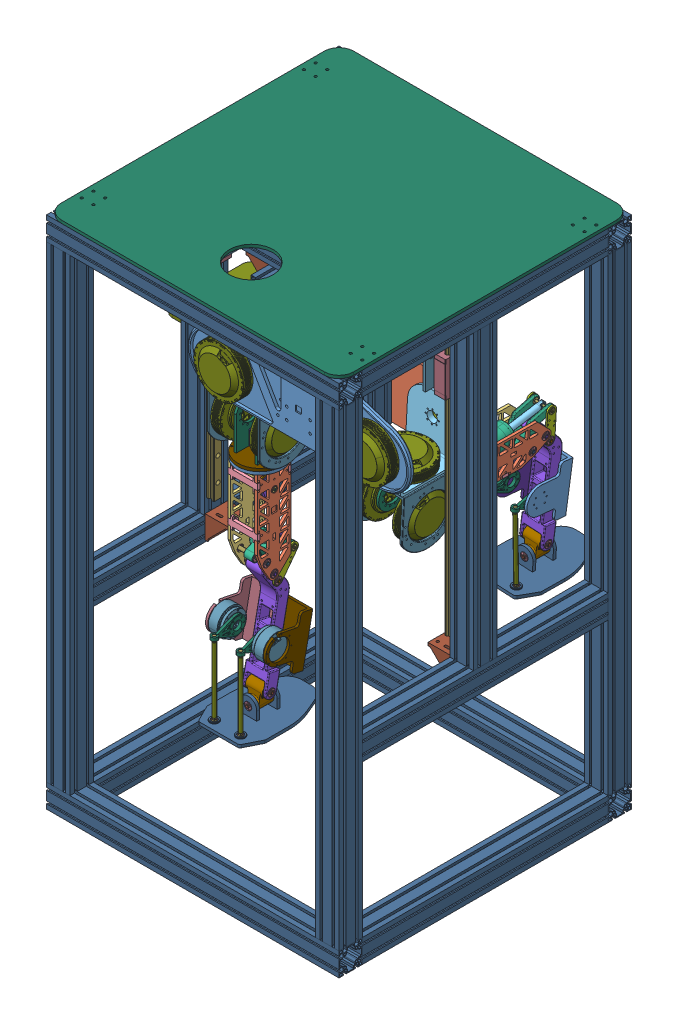
SolidWorks assembly 完整下肢, configuration 默认. Lengths in mm. (continued)
Mates (geometry in assembly coordinates): (continued)
- 同心162: concentric anti-aligned: cylinder of 脚踝十字连接-1 through (-301.8233 -1070.6139 623.2525) axis (0 0 1) radius 11; cylinder of 轴承_NSK6900NR-39 through (-301.8233 -1070.6139 624.6412) axis (0 0 -1) radius 11
- 重合185: coincident anti-aligned: plane of 脚踝十字连接-1 through (-301.8233 -1070.6139 625.0025) normal (0 0 -1); plane of 轴承_NSK6900NR-39 through (-301.8233 -1070.6139 625.0025) normal (0 0 1)
- 同心163: concentric aligned: cylinder of 脚踝十字连接-1 through (-301.8233 -1070.6139 623.2525) axis (0 0 1) radius 11; cylinder of 轴承_NSK6900NR-40 through (-301.8233 -1070.6139 679.8638) axis (0 0 1) radius 11
- 重合186: coincident anti-aligned: plane of 脚踝十字连接-1 through (-301.8233 -1070.6139 679.5025) normal (0 0 1); plane of 轴承_NSK6900NR-40 through (-301.8233 -1070.6139 679.5025) normal (0 0 -1)
- 同心164: concentric anti-aligned: cylinder of 脚踝十字连接-2 through (165.9433 -632.5913 204.3739) axis (-0.000652 -0.012197 -0.999925) radius 11; cylinder of 轴承_NSK6900NR-41 through (165.9424 -632.6083 202.9853) axis (0.000652 0.012197 0.999925) radius 11
- 重合187: coincident anti-aligned: plane of 脚踝十字连接-2 through (165.9422 -632.6127 202.624) normal (0.000652 0.012197 0.999925); plane of 轴承_NSK6900NR-41 through (165.9422 -632.6127 202.624) normal (-0.000652 -0.012197 -0.999925)
- 同心165: concentric aligned: cylinder of 脚踝十字连接-2 through (139.0993 -591.458 174.8875) axis (0.998576 -0.053343 0) radius 11; cylinder of 轴承_NSK6900NR-42 through (195.63 -594.4778 174.8875) axis (0.998576 -0.053343 0) radius 11
- 重合188: coincident anti-aligned: plane of 脚踝十字连接-2 through (195.2692 -594.4586 174.8875) normal (0.998576 -0.053343 0); plane of 轴承_NSK6900NR-42 through (195.2692 -594.4586 174.8875) normal (-0.998576 0.053343 0)
- 同心166: concentric anti-aligned: cylinder of 脚踝十字连接-2 through (139.0993 -591.458 174.8875) axis (0.998576 -0.053343 0) radius 11; cylinder of 轴承_NSK6900NR-43 through (140.486 -591.5321 174.8875) axis (-0.998576 0.053343 0) radius 11
- 重合189: coincident anti-aligned: plane of 脚踝十字连接-2 through (140.8468 -591.5514 174.8875) normal (-0.998576 0.053343 0); plane of 轴承_NSK6900NR-43 through (140.8468 -591.5514 174.8875) normal (0.998576 -0.053343 0)
- 同心167: concentric aligned: cylinder of 脚踝十字连接-2 through (165.9433 -632.5913 204.3739) axis (-0.000652 -0.012197 -0.999925) radius 11; cylinder of 轴承_NSK6900NR-44 through (165.9064 -633.2818 147.7668) axis (-0.000652 -0.012197 -0.999925) radius 11
- 重合191: coincident anti-aligned: plane of 脚踝十字连接-2 through (165.9067 -633.2774 148.1281) normal (-0.000652 -0.012197 -0.999925); plane of 轴承_NSK6900NR-44 through (165.9067 -633.2774 148.1281) normal (0.000652 0.012197 0.999925)
- 同心168: concentric aligned: cylinder of 轴承_NSK6900NR-34 through (207.6129 -595.1179 174.8875) axis (0.998576 -0.053343 0) radius 5; cylinder of 踝关节轴-1 through (211.9953 -595.3521 174.8875) axis (0.998576 -0.053343 0) radius 5
- 距离13: distance = 3 mm aligned: plane of 踝关节轴-1 through (123.8757 -595.243 176.8665) normal (-0.998576 0.053343 0); plane of 轴承_NSK6900NR-36 through (126.77 -597.3018 174.5884) normal (-0.998576 0.053343 0)
- 同心169: concentric anti-aligned: cylinder of 轴承_NSK6900NR-33 through (-341.4346 -1030.6139 652.2525) axis (-1 0 0) radius 5; cylinder of 踝关节轴-2 through (-257.8233 -1030.6139 652.2525) axis (1 0 0) radius 5
- 距离14: distance = 3 mm aligned: plane of 踝关节轴-2 through (-345.8233 -1035.6049 651.9533) normal (-1 0 0); plane of 轴承_NSK6900NR-33 through (-342.8233 -1036.7707 654.3365) normal (-1 0 0)
- 同心170: concentric aligned: cylinder of 轴承_NSK6900NR-42 through (195.63 -594.4778 174.8875) axis (0.998576 -0.053343 0) radius 5; cylinder of 踝关节轴-1 through (211.9953 -595.3521 174.8875) axis (0.998576 -0.053343 0) radius 5
- 同心171: concentric anti-aligned: cylinder of 轴承_NSK6900NR-37 through (-329.4346 -1030.6139 652.2525) axis (-1 0 0) radius 5; cylinder of 踝关节轴-2 through (-257.8233 -1030.6139 652.2525) axis (1 0 0) radius 5
- 同心172: concentric anti-aligned: cylinder of 踝关节轴-2 through (-257.8233 -1030.6139 652.2525) axis (1 0 0) radius 5; cylinder of 轴套V2-2 through (-330.8233 -1030.6139 652.2525) axis (-1 0 0) radius 5
- 同心173: concentric anti-aligned: cylinder of 踝关节轴-2 through (-257.8233 -1030.6139 652.2525) axis (1 0 0) radius 5; cylinder of 轴套V2-1 through (-266.8233 -1030.6139 652.2525) axis (-1 0 0) radius 5
- 同心174: concentric aligned: cylinder of 踝关节轴-1 through (211.9953 -595.3521 174.8875) axis (0.998576 -0.053343 0) radius 5; cylinder of 轴套V2-4 through (197.0167 -594.5519 174.8875) axis (0.998576 -0.053343 0) radius 5
- 同心175: concentric aligned: cylinder of 踝关节轴-1 through (211.9953 -595.3521 174.8875) axis (0.998576 -0.053343 0) radius 5; cylinder of 轴套V2-3 through (133.1078 -591.138 174.8875) axis (0.998576 -0.053343 0) radius 5
- 重合194: coincident anti-aligned: plane of 轴承_NSK6900NR-42 through (197.1356 -592.3254 180.9931) normal (0.998576 -0.053343 0); plane of 轴套V2-4 through (197.0167 -594.5519 174.8875) normal (-0.998576 0.053343 0)
- 重合195: coincident anti-aligned: plane of 轴承_NSK6900NR-43 through (139.0705 -591.9972 181.365) normal (-0.998576 0.053343 0); plane of 轴套V2-3 through (139.0993 -591.458 174.8875) normal (0.998576 -0.053343 0)
- 重合196: coincident anti-aligned: plane of 轴承_NSK6900NR-36 through (132.8414 -596.1256 174.6574) normal (0.998576 -0.053343 0); plane of 轴套V2-3 through (133.1078 -591.138 174.8875) normal (-0.998576 0.053343 0)
- 重合197: coincident anti-aligned: plane of 轴承_NSK6900NR-38 through (-272.8233 -1031.6087 645.8291) normal (1 0 0); plane of 轴套V2-1 through (-272.8233 -1030.6139 652.2525) normal (-1 0 0)
- 重合198: coincident anti-aligned: plane of 轴承_NSK6900NR-37 through (-330.8233 -1032.1555 658.567) normal (-1 0 0); plane of 轴套V2-2 through (-330.8233 -1030.6139 652.2525) normal (1 0 0)
- 重合199: coincident anti-aligned: plane of 轴承_NSK6900NR-33 through (-336.8233 -1035.3499 653.8556) normal (1 0 0); plane of 轴套V2-2 through (-336.8233 -1030.6139 652.2525) normal (-1 0 0)
- 同心176: concentric aligned: cylinder of 球铰脚底板-1 through (-301.8233 -1070.6139 612.2525) axis (0 0 1) radius 11; cylinder of 轴承_NSK6900NR-45 through (-301.8233 -1070.6139 691.8638) axis (0 0 1) radius 11
- 重合200: coincident anti-aligned: plane of 球铰脚底板-1 through (-301.8233 -1070.6139 691.5025) normal (0 0 1); plane of 轴承_NSK6900NR-45 through (-301.8233 -1070.6139 691.5025) normal (0 0 -1)
- 同心177: concentric anti-aligned: cylinder of 球铰脚底板-1 through (-301.8233 -1070.6139 612.2525) axis (0 0 1) radius 11; cylinder of 轴承_NSK6900NR-46 through (-301.8233 -1070.6139 612.6412) axis (0 0 -1) radius 11
- 重合201: coincident anti-aligned: plane of 球铰脚底板-1 through (-301.8233 -1070.6139 613.0025) normal (0 0 -1); plane of 轴承_NSK6900NR-46 through (-301.8233 -1070.6139 613.0025) normal (0 0 1)
- 同心178: concentric aligned: cylinder of 球铰脚底板-2 through (165.8984 -633.4329 135.379) axis (0.000652 0.012197 0.999925) radius 11; cylinder of 轴承_NSK6900NR-47 through (165.9502 -632.4619 214.9844) axis (0.000652 0.012197 0.999925) radius 11
- 重合202: coincident anti-aligned: plane of 球铰脚底板-2 through (165.95 -632.4663 214.6231) normal (0.000652 0.012197 0.999925); plane of 轴承_NSK6900NR-47 through (165.95 -632.4663 214.6231) normal (-0.000652 -0.012197 -0.999925)
- 同心179: concentric anti-aligned: cylinder of 球铰脚底板-2 through (165.8984 -633.4329 135.379) axis (0.000652 0.012197 0.999925) radius 11; cylinder of 轴承_NSK6900NR-48 through (165.8986 -633.4282 135.7677) axis (-0.000652 -0.012197 -0.999925) radius 11
- 重合203: coincident anti-aligned: plane of 球铰脚底板-2 through (165.8989 -633.4238 136.129) normal (-0.000652 -0.012197 -0.999925); plane of 轴承_NSK6900NR-48 through (165.8989 -633.4238 136.129) normal (0.000652 0.012197 0.999925)
- 同心180: concentric anti-aligned: cylinder of 轴承_NSK6900NR-47 through (165.9502 -632.4619 214.9844) axis (0.000652 0.012197 0.999925) radius 5; cylinder of 踝关节轴-4 through (165.8958 -633.4817 131.3793) axis (-0.000652 -0.012197 -0.999925) radius 5
- 距离15: distance = 3 mm aligned: plane of 踝关节轴-4 through (170.4943 -634.5004 219.3953) normal (0.000652 0.012197 0.999925); plane of 轴承_NSK6900NR-47 through (159.456 -632.194 216.3742) normal (0.000652 0.012197 0.999925)
- 同心181: concentric anti-aligned: cylinder of 轴承_NSK6900NR-45 through (-301.8233 -1070.6139 691.8638) axis (0 0 1) radius 5; cylinder of 踝关节轴-3 through (-301.8233 -1070.6139 608.2525) axis (0 0 -1) radius 5
- 距离16: distance = 3 mm aligned: plane of 踝关节轴-3 through (-296.8235 -1070.5647 696.2525) normal (0 0 1); plane of 轴承_NSK6900NR-45 through (-307.8028 -1073.1626 693.2525) normal (0 0 1)
- 重合206: coincident anti-aligned: plane of 轴承_NSK6900NR-45 through (-306.4229 -1072.5744 687.2525) normal (0 0 -1); plane of 轴套-27 through (-301.8233 -1070.6139 687.2525) normal (0 0 1)
- 同心182: concentric aligned: cylinder of 踝关节轴-3 through (-301.8233 -1070.6139 608.2525) axis (0 0 -1) radius 5; cylinder of 轴套-27 through (-301.8233 -1070.6139 687.2525) axis (0 0 -1) radius 5
- 同心183: concentric aligned: cylinder of 踝关节轴-3 through (-301.8233 -1070.6139 608.2525) axis (0 0 -1) radius 5; cylinder of 轴套-28 through (-301.8233 -1070.6139 623.2525) axis (0 0 -1) radius 5
- 重合207: coincident anti-aligned: plane of 轴承_NSK6900NR-46 through (-296.8235 -1070.5647 617.2525) normal (0 0 1); plane of 轴套-28 through (-301.8233 -1070.6139 617.2525) normal (0 0 -1)
- 同心184: concentric aligned: cylinder of 踝关节轴-4 through (165.8958 -633.4817 131.3793) axis (-0.000652 -0.012197 -0.999925) radius 5; cylinder of 轴套-29 through (165.9055 -633.2988 146.3782) axis (-0.000652 -0.012197 -0.999925) radius 5
- 重合208: coincident anti-aligned: plane of 轴承_NSK6900NR-48 through (170.4429 -635.464 140.4012) normal (0.000652 0.012197 0.999925); plane of 轴套-29 through (165.9016 -633.3719 140.3787) normal (-0.000652 -0.012197 -0.999925)
- 同心185: concentric aligned: cylinder of 踝关节轴-4 through (165.8958 -633.4817 131.3793) axis (-0.000652 -0.012197 -0.999925) radius 5; cylinder of 轴套-30 through (165.9472 -632.5182 210.3734) axis (-0.000652 -0.012197 -0.999925) radius 5
- 重合209: coincident anti-aligned: plane of 轴承_NSK6900NR-47 through (160.951 -632.3251 210.3743) normal (-0.000652 -0.012197 -0.999925); plane of 轴套-30 through (165.9472 -632.5182 210.3734) normal (0.000652 0.012197 0.999925)
- 重合210: coincident anti-aligned: plane of 轴承_NSK6900NR-41 through (171.2206 -636.3859 204.4167) normal (0.000652 0.012197 0.999925); plane of 轴套-30 through (165.9433 -632.5913 204.3739) normal (-0.000652 -0.012197 -0.999925)
- 同心186: concentric anti-aligned: cylinder of 轴承_NSK6900NR-41 through (165.9424 -632.6083 202.9853) axis (0.000652 0.012197 0.999925) radius 5; cylinder of 踝关节轴-4 through (165.8958 -633.4817 131.3793) axis (-0.000652 -0.012197 -0.999925) radius 5
- 重合211: coincident anti-aligned: plane of 轴承_NSK6900NR-40 through (-307.0386 -1074.4934 681.2525) normal (0 0 1); plane of 轴套-27 through (-301.8233 -1070.6139 681.2525) normal (0 0 -1)
- 同心187: concentric anti-aligned: cylinder of 轴承_NSK6900NR-40 through (-301.8233 -1070.6139 679.8638) axis (0 0 1) radius 5; cylinder of 踝关节轴-3 through (-301.8233 -1070.6139 608.2525) axis (0 0 -1) radius 5
- 重合212: coincident anti-aligned: plane of 球铰脚底板-1 through (-301.8233 -1106.6139 792.2525) normal (0 1 0); plane of 关节轴承外圈_SQD6-4 through (-342.3507 -1106.6139 766.4483) normal (0 -1 0)
- 同心188: concentric aligned: cylinder of 球铰脚底板-1 through (-346.8233 -1136.0697 762.2525) axis (0 1 0) radius 9; cylinder of 关节轴承外圈_SQD6-4 through (-346.8233 -1094.8853 762.2525) axis (0 1 0) radius 9
- 重合213: coincident anti-aligned: plane of 球铰脚底板-1 through (-301.8233 -1106.6139 792.2525) normal (0 1 0); plane of 关节轴承外圈_SQD6-3 through (-252.3507 -1106.6139 766.4483) normal (0 -1 0)
- 同心189: concentric aligned: cylinder of 球铰脚底板-1 through (-256.8233 -1136.0697 762.2525) axis (0 1 0) radius 9; cylinder of 关节轴承外圈_SQD6-3 through (-256.8233 -1094.8853 762.2525) axis (0 1 0) radius 9
- 重合214: coincident anti-aligned: plane of 球铰脚底板-2 through (164.0955 -667.1835 315.8053) normal (0.053339 0.998502 -0.012214); plane of 关节轴承外圈_SQD6-2 through (125.2636 -665.4768 285.7544) normal (-0.053339 -0.998502 0.012214)
- 同心190: concentric aligned: cylinder of 球铰脚底板-2 through (117.5688 -694.5607 286.1673) axis (0.053339 0.998502 -0.012214) radius 9; cylinder of 关节轴承外圈_SQD6-2 through (119.7656 -653.438 285.6643) axis (0.053339 0.998502 -0.012214) radius 9
- 重合215: coincident anti-aligned: plane of 球铰脚底板-2 through (164.0955 -667.1835 315.8053) normal (0.053339 0.998502 -0.012214); plane of 关节轴承外圈_SQD6-1 through (215.1355 -670.2776 285.7544) normal (-0.053339 -0.998502 0.012214)
- 同心191: concentric aligned: cylinder of 球铰脚底板-2 through (207.4407 -699.3616 286.1673) axis (0.053339 0.998502 -0.012214) radius 9; cylinder of 关节轴承外圈_SQD6-1 through (209.6374 -658.2389 285.6643) axis (0.053339 0.998502 -0.012214) radius 9
- 同心192: concentric: sphere of 关节轴承外圈_SQD6-1; unknown of 关节轴承内杆_SQD6-4
- 同心193: concentric: unknown of 关节轴承外圈_SQD6-2; unknown of 关节轴承内杆_SQD6-3
- 同心194: concentric: unknown of 关节轴承外圈_SQD6-3; unknown of 关节轴承内杆_SQD6-2
- 同心195: concentric: unknown of 关节轴承外圈_SQD6-4; unknown of 关节轴承内杆_SQD6-1
- 重合216: coincident anti-aligned: plane of 小腿主干-2 through (-331.8233 -751.8502 576.1037) normal (0 -0.196116 -0.980581); plane of 小腿左侧电机安装板A1-1 through (-295.3233 -955.1042 616.7545) normal (0 0.196116 0.980581)
- 同心196: concentric aligned: cylinder of 小腿主干-2 through (-320.3233 -786.4443 695.2009) axis (0 -0.196116 -0.980581) radius 2.75; cylinder of 小腿左侧电机安装板A1-1 through (-320.3233 -799.7802 628.5214) axis (0 -0.196116 -0.980581) radius 2.75
- 同心197: concentric aligned: cylinder of 小腿主干-2 through (-320.3233 -913.9198 720.696) axis (0 -0.196116 -0.980581) radius 2.75; cylinder of 小腿左侧电机安装板A1-1 through (-320.3233 -927.2557 654.0165) axis (0 -0.196116 -0.980581) radius 2.75
- 重合218: coincident anti-aligned: plane of 小腿左侧电机安装板A1-1 through (-396.8233 -788.4055 583.4147) normal (1 0 0); plane of A1电机-1 through (-396.8233 -854.1044 688.3369) normal (-1 0 0)
- 同心200: concentric anti-aligned: cylinder of 小腿左侧电机安装板A1-1 through (-576.8233 -854.1044 688.3369) axis (1 0 0) radius 46; cylinder of A1电机-1 through (-364.8233 -854.1044 688.3369) axis (-1 0 0) radius 46
- 重合223: coincident anti-aligned: plane of 小腿主干-2 through (-301.8233 -673.6825 652.2525) normal (1 0 0); plane of 球铰脚底板-1 through (-301.8233 -1110.6139 792.2525) normal (-1 0 0)
- 同心202: concentric anti-aligned: cylinder of A1电机-1 through (-353.8233 -854.1044 688.3369) axis (1 0 0) radius 26.5; cylinder of 小腿电机摇杆A1-1 through (-341.8233 -854.1044 688.3369) axis (-1 0 0) radius 26.5
- 重合224: coincident anti-aligned: plane of A1电机-1 through (-351.8233 -854.1044 688.3369) normal (1 0 0); plane of 小腿电机摇杆A1-1 through (-351.8233 -854.1044 688.3369) normal (-1 0 0)
- 同心204: concentric anti-aligned: cylinder of 小腿电机摇杆A1-1 through (-346.8233 -823.0582 762.1623) axis (0 -0.999996 0.002916) radius 9; cylinder of 关节轴承外圈_SQD6-5 through (-346.8233 -845.5353 762.2278) axis (0 0.999996 -0.002916) radius 9
- 重合226: coincident anti-aligned: plane of 小腿电机摇杆A1-1 through (-346.8233 -850.546 751.2424) normal (0 -0.999996 0.002916); plane of 关节轴承外圈_SQD6-5 through (-340.7094 -850.5153 761.7634) normal (0 0.999996 -0.002916)
- 同心205: concentric: unknown of 关节轴承外圈_SQD6-5; unknown of 关节轴承内杆_SQD6-5
- 同心206: concentric anti-aligned: cylinder of 关节轴承内杆_SQD6-1 through (-346.8233 -1073.0639 762.2524) axis (0 1 -0.000001) radius 3; cylinder of 关节轴承内杆_SQD6-5 through (-346.8233 -884.0639 762.2522) axis (0 -1 0.000001) radius 3
- 平行11: parallel aligned: plane of 小腿主干-2 through (-271.8233 -673.6825 652.2525) normal (0 0 1); plane of 球铰脚底板-1 through (-401.8233 -1100.6139 792.2525) normal (0 0 1)
- 同心207: concentric aligned: cylinder of 关节轴承内杆_SQD6-5 through (-346.8233 -884.0639 762.2522) axis (0 -1 0.000001) radius 3; cylinder of 踝关节连杆-1 through (-346.8233 -866.0639 762.2522) axis (0 -1 0.000001) radius 3
- 同心208: concentric anti-aligned: cylinder of 关节轴承内杆_SQD6-1 through (-346.8233 -1073.0639 762.2524) axis (0 1 -0.000001) radius 3; cylinder of 踝关节连杆-1 through (-346.8233 -866.0639 762.2522) axis (0 -1 0.000001) radius 3
- 重合230: coincident anti-aligned: plane of 关节轴承内杆_SQD6-1 through (-341.8309 -1091.0639 761.9761) normal (0 1 -0.000001); plane of 踝关节连杆-1 through (-346.8233 -1091.0639 762.2525) normal (0 -1 0.000001)
- 重合231: coincident anti-aligned: plane of 关节轴承内杆_SQD6-5 through (-351.6226 -866.0639 760.8497) normal (0 -1 0.000001); plane of 踝关节连杆-1 through (-346.8233 -866.0639 762.2522) normal (0 1 -0.000001)
- 同心209: concentric aligned: cylinder of 小腿左侧电机安装板A1-1 through (-394.8233 -812.4297 680.0019) axis (-1 0 0) radius 1.75; cylinder of A1电机-1 through (-390.8233 -812.4297 680.0019) axis (-1 0 0) radius 1.5
- 重合232: coincident anti-aligned: plane of 小腿主干-1 through (153.3145 -306.6032 128.3635) normal (-0.004924 -0.092171 -0.995731); plane of 小腿左侧定脚踝安装板-1 through (178.7528 -514.6507 147.4959) normal (0.004924 0.092171 0.995731)
- 同心210: concentric aligned: cylinder of 小腿主干-1 through (162.2973 -354.0313 243.1809) axis (-0.004924 -0.092171 -0.995731) radius 2.75; cylinder of 小腿左侧定脚踝安装板-1 through (161.9625 -360.299 175.4712) axis (-0.004924 -0.092171 -0.995731) radius 2.75
- 同心211: concentric aligned: cylinder of 小腿主干-1 through (155.3923 -483.2921 255.1802) axis (-0.004924 -0.092171 -0.995731) radius 2.75; cylinder of 小腿左侧定脚踝安装板-1 through (155.0575 -489.5597 187.4705) axis (-0.004924 -0.092171 -0.995731) radius 2.75
- 重合233: coincident anti-aligned: plane of 小腿左侧定脚踝安装板-1 through (131.3628 -342.6036 131.8044) normal (0.998576 -0.053343 0); plane of 小腿电机摇杆A1-3 through (127.2912 -418.8248 229.2659) normal (-0.998576 0.053343 0)
- 重合234: coincident anti-aligned: plane of 小腿电机摇杆A1-3 through (132.7234 -410.8671 291.7314) normal (-0.053183 -0.995579 0.077426); plane of 关节轴承外圈_SQD6-6 through (131.6567 -410.4252 296.6813) normal (0.053183 0.995579 -0.077426)
- 同心216: concentric aligned: cylinder of 小腿电机摇杆A1-3 through (134.229 -382.6822 300.5726) axis (-0.053183 -0.995579 0.077426) radius 9; cylinder of 关节轴承外圈_SQD6-6 through (132.1451 -421.6934 303.6065) axis (-0.053183 -0.995579 0.077426) radius 9
- 同心217: concentric: unknown of 关节轴承内杆_SQD6-6; unknown of 关节轴承外圈_SQD6-6
- 同心218: concentric anti-aligned: cylinder of 关节轴承内杆_SQD6-6 through (130.9836 -443.437 300.879) axis (-0.053216 -0.9962 -0.068953) radius 3; cylinder of 踝关节连杆-2 through (119.9679 -649.6504 286.6058) axis (0.053216 0.9962 0.068953) radius 3
- 重合235: coincident anti-aligned: plane of 关节轴承内杆_SQD6-6 through (133.1138 -425.9034 306.9645) normal (-0.053216 -0.9962 -0.068953); plane of 踝关节连杆-2 through (131.9415 -425.5054 302.1202) normal (0.053216 0.9962 0.068953)
- 同心219: concentric aligned: cylinder of 关节轴承内杆_SQD6-3 through (120.9258 -631.7188 287.847) axis (0.053216 0.9962 0.068953) radius 3; cylinder of 踝关节连杆-2 through (119.9679 -649.6504 286.6058) axis (0.053216 0.9962 0.068953) radius 3
- 重合237: coincident anti-aligned: plane of 关节轴承内杆_SQD6-3 through (123.5072 -650.082 290.1111) normal (0.053216 0.9962 0.068953); plane of 踝关节连杆-2 through (119.9679 -649.6504 286.6058) normal (-0.053216 -0.9962 -0.068953)
- 重合239: coincident anti-aligned: plane of 小腿电机摇杆A1-4 through (222.5953 -415.668 291.7314) normal (-0.053183 -0.995579 0.077426); plane of 关节轴承外圈_SQD6-8 through (216.556 -414.5482 301.9819) normal (0.053183 0.995579 -0.077426)
- 同心220: concentric aligned: cylinder of 小腿电机摇杆A1-4 through (224.1009 -387.483 300.5726) axis (-0.053183 -0.995579 0.077426) radius 9; cylinder of 关节轴承外圈_SQD6-8 through (222.017 -426.4942 303.6065) axis (-0.053183 -0.995579 0.077426) radius 9
- 同心221: concentric: unknown of 关节轴承内杆_SQD6-8; unknown of 关节轴承外圈_SQD6-8
- 同心222: concentric anti-aligned: cylinder of 关节轴承内杆_SQD6-4 through (210.7976 -636.5196 287.847) axis (0.053216 0.9962 0.068953) radius 3; cylinder of 关节轴承内杆_SQD6-8 through (220.8554 -448.2379 300.879) axis (-0.053216 -0.9962 -0.068953) radius 3
- 同心223: concentric aligned: cylinder of 关节轴承内杆_SQD6-8 through (220.8554 -448.2379 300.879) axis (-0.053216 -0.9962 -0.068953) radius 3; cylinder of 踝关节连杆-4 through (221.8133 -430.3063 302.1202) axis (-0.053216 -0.9962 -0.068953) radius 3
- 重合240: coincident anti-aligned: plane of 关节轴承内杆_SQD6-8 through (226.7853 -430.6022 302.5586) normal (-0.053216 -0.9962 -0.068953); plane of 踝关节连杆-4 through (221.8133 -430.3063 302.1202) normal (0.053216 0.9962 0.068953)
- 重合241: coincident anti-aligned: plane of 关节轴承内杆_SQD6-4 through (214.8318 -654.71 286.4917) normal (0.053216 0.9962 0.068953); plane of 踝关节连杆-4 through (209.8398 -654.4512 286.6058) normal (-0.053216 -0.9962 -0.068953)
- 重合242: coincident anti-aligned: plane of 镜向小腿左侧电机安装板A1-3 through (-206.8233 -788.4055 583.4147) normal (-1 0 0); plane of A1电机-3 through (-206.8233 -854.1044 688.3369) normal (1 0 0)
- 同心224: concentric anti-aligned: cylinder of 镜向小腿左侧电机安装板A1-3 through (-26.8233 -854.1044 688.3369) axis (-1 0 0) radius 46; cylinder of A1电机-3 through (-238.8233 -854.1044 688.3369) axis (1 0 0) radius 46
- 同心225: concentric aligned: cylinder of 镜向小腿左侧电机安装板A1-3 through (-208.8233 -818.7423 711.9116) axis (1 0 0) radius 1.75; cylinder of A1电机-3 through (-212.8233 -818.7423 711.9116) axis (1 0 0) radius 1.5
- 重合243: coincident anti-aligned: plane of 小腿电机摇杆A1-5 through (-251.8233 -854.1044 688.3369) normal (1 0 0); plane of A1电机-3 through (-251.8233 -854.1044 688.3369) normal (-1 0 0)
- 重合244: coincident anti-aligned: plane of 小腿电机摇杆A1-5 through (-256.8233 -850.546 751.2424) normal (0 -0.999996 0.002916); plane of 关节轴承外圈_SQD6-9 through (-250.8756 -850.5095 763.7372) normal (0 0.999996 -0.002916)
- 同心228: concentric anti-aligned: cylinder of 小腿电机摇杆A1-5 through (-256.8233 -823.0582 762.1623) axis (0 -0.999996 0.002916) radius 9; cylinder of 关节轴承外圈_SQD6-9 through (-256.8233 -845.5353 762.2278) axis (0 0.999996 -0.002916) radius 9
- 同心229: concentric: unknown of 关节轴承内杆_SQD6-9; unknown of 关节轴承外圈_SQD6-9
- 同心230: concentric anti-aligned: cylinder of 关节轴承内杆_SQD6-9 through (-256.8233 -884.0639 762.2522) axis (0 -1 0.000001) radius 3; cylinder of 踝关节连杆-5 through (-256.8233 -1091.0639 762.2525) axis (0 1 -0.000001) radius 3
- 同心231: concentric aligned: cylinder of 关节轴承内杆_SQD6-2 through (-256.8233 -1073.0639 762.2524) axis (0 1 -0.000001) radius 3; cylinder of 踝关节连杆-5 through (-256.8233 -1091.0639 762.2525) axis (0 1 -0.000001) radius 3
- 重合245: coincident anti-aligned: plane of 关节轴承内杆_SQD6-2 through (-251.8329 -1091.0639 761.9424) normal (0 1 -0.000001); plane of 踝关节连杆-5 through (-256.8233 -1091.0639 762.2525) normal (0 -1 0.000001)
- 同心232: concentric anti-aligned: cylinder of 小腿电机摇杆A1-5 through (-256.8233 -854.1044 688.3369) axis (1 0 0) radius 30; cylinder of A1电机-3 through (-249.8233 -854.1044 688.3369) axis (-1 0 0) radius 26.5
- 重合246: coincident anti-aligned: plane of 关节轴承内杆_SQD6-9 through (-251.9673 -866.0639 761.0609) normal (0 -1 0.000001); plane of 踝关节连杆-5 through (-256.8233 -866.0639 762.2522) normal (0 1 -0.000001)
- 重合251: coincident anti-aligned: plane of 大腿_电机轴-1 through (136.2219 -232.8956 462.2655) normal (-0.998576 0.053343 0); plane of 轴用挡圈GB894-5-1 through (136.2152 -233.0212 461.8858) normal (0.998576 -0.053343 0)
- 同心237: concentric anti-aligned: cylinder of 大腿_电机轴-1 through (133.2262 -232.7356 462.2655) axis (0.998576 -0.053343 0) radius 2.5; cylinder of 轴用挡圈GB894-5-1 through (136.2219 -232.8956 462.2655) axis (-0.998576 0.053343 0) radius 2.35
- 重合252: coincident anti-aligned: plane of 大腿_电机轴-2 through (-352.8233 -423.6825 652.2525) normal (-1 0 0); plane of 轴用挡圈GB894-5-2 through (-352.8233 -423.7044 651.8531) normal (1 0 0)
- 同心238: concentric aligned: cylinder of 大腿_电机轴-2 through (-355.8233 -423.6825 652.2525) axis (1 0 0) radius 2.5; cylinder of 轴用挡圈GB894-5-2 through (-353.3233 -423.6825 652.2525) axis (1 0 0) radius 2.35
- 重合253: coincident anti-aligned: plane of 大腿_电机轴-2 through (-250.8233 -423.6825 652.2525) normal (1 0 0); plane of 轴用挡圈GB894-5-3 through (-250.8233 -423.7044 651.8531) normal (-1 0 0)
- 同心239: concentric aligned: cylinder of 大腿_电机轴-2 through (-355.8233 -423.6825 652.2525) axis (1 0 0) radius 2.5; cylinder of 轴用挡圈GB894-5-3 through (-250.8233 -423.6825 652.2525) axis (1 0 0) radius 2.35
- 重合254: coincident anti-aligned: plane of 大腿_电机轴-1 through (238.0767 -238.3366 462.2655) normal (0.998576 -0.053343 0); plane of 轴用挡圈GB894-5-4 through (238.0793 -238.2875 462.6625) normal (-0.998576 0.053343 0)
- 同心240: concentric aligned: cylinder of 大腿_电机轴-1 through (133.2262 -232.7356 462.2655) axis (0.998576 -0.053343 0) radius 2.5; cylinder of 轴用挡圈GB894-5-4 through (238.0767 -238.3366 462.2655) axis (0.998576 -0.053343 0) radius 2.35
- 重合255: coincident anti-aligned: plane of 上下连杆轴-2 through (-264.8233 -643.2766 570.5287) normal (1 0 0); plane of 轴用挡圈GB894-5-5 through (-264.8233 -643.2985 570.1293) normal (-1 0 0)
- 同心241: concentric anti-aligned: cylinder of 上下连杆轴-2 through (-261.8233 -643.2766 570.5287) axis (-1 0 0) radius 2.5; cylinder of 轴用挡圈GB894-5-5 through (-264.8233 -643.2766 570.5287) axis (1 0 0) radius 2.35
- 重合256: coincident anti-aligned: plane of 上下连杆轴-1 through (226.689 -189.0594 179.8677) normal (0.998576 -0.053343 0); plane of 轴用挡圈GB894-5-6 through (226.6917 -189.0103 180.2647) normal (-0.998576 0.053343 0)
- 同心242: concentric aligned: cylinder of 上下连杆轴-1 through (149.7987 -184.952 179.8677) axis (0.998576 -0.053343 0) radius 2.5; cylinder of 轴用挡圈GB894-5-6 through (226.689 -189.0594 179.8677) axis (0.998576 -0.053343 0) radius 2.35
- 重合257: coincident anti-aligned: plane of 上下连杆轴-1 through (152.7944 -185.112 179.8677) normal (-0.998576 0.053343 0); plane of 轴用挡圈GB894-5-7 through (152.7877 -185.2377 179.488) normal (0.998576 -0.053343 0)
- 同心243: concentric anti-aligned: cylinder of 上下连杆轴-1 through (149.7987 -184.952 179.8677) axis (0.998576 -0.053343 0) radius 2.5; cylinder of 轴用挡圈GB894-5-7 through (152.7944 -185.112 179.8677) axis (-0.998576 0.053343 0) radius 2.35
- 重合258: coincident anti-aligned: plane of 上下连杆轴-2 through (-338.8233 -643.2766 570.5287) normal (-1 0 0); plane of 轴用挡圈GB894-5-8 through (-338.8233 -642.8836 570.6033) normal (1 0 0)
- 同心244: concentric aligned: cylinder of 上下连杆轴-2 through (-261.8233 -643.2766 570.5287) axis (-1 0 0) radius 2.5; cylinder of 轴用挡圈GB894-5-8 through (-338.8233 -643.2766 570.5287) axis (-1 0 0) radius 2.35
- 重合259: coincident anti-aligned: plane of 上连杆大腿轴-1 through (-352.8233 -630.3812 677.2525) normal (-1 0 0); plane of 轴用挡圈GB894-10-5 through (-352.8233 -629.6935 677.383) normal (1 0 0)
- 同心245: concentric aligned: cylinder of 上连杆大腿轴-1 through (-355.8233 -630.3812 677.2525) axis (-1 0 0) radius 5; cylinder of 轴用挡圈GB894-10-5 through (-352.8233 -630.3812 677.2525) axis (-1 0 0) radius 4.65
- 重合260: coincident anti-aligned: plane of 大腿小腿轴-2 through (-352.8233 -673.6825 652.2525) normal (-1 0 0); plane of 轴用挡圈GB894-10-6 through (-352.8233 -672.9948 652.383) normal (1 0 0)
- 同心246: concentric aligned: cylinder of 大腿小腿轴-2 through (-355.8233 -673.6825 652.2525) axis (-1 0 0) radius 5; cylinder of 轴用挡圈GB894-10-6 through (-352.8233 -673.6825 652.2525) axis (-1 0 0) radius 4.65
- 重合261: coincident anti-aligned: plane of 下连杆小腿轴-2 through (-338.8233 -715.285 624.5175) normal (-1 0 0); plane of 轴用挡圈GB894-10-7 through (-338.8233 -714.5973 624.648) normal (1 0 0)
- 同心247: concentric aligned: cylinder of 下连杆小腿轴-2 through (-341.8233 -715.285 624.5175) axis (-1 0 0) radius 5; cylinder of 轴用挡圈GB894-10-7 through (-338.8233 -715.285 624.5175) axis (-1 0 0) radius 4.65
- 重合262: coincident anti-aligned: plane of 上连杆大腿轴-2 through (134.7591 -260.2785 255.8742) normal (-0.998576 0.053343 0); plane of 轴用挡圈GB894-10-8 through (134.7474 -260.4984 255.2097) normal (0.998576 -0.053343 0)
- 重合263: coincident anti-aligned: plane of 大腿小腿轴-1 through (136.0655 -235.8228 212.2827) normal (-0.998576 0.053343 0); plane of 轴用挡圈GB894-10-9 through (136.0538 -236.0427 211.6183) normal (0.998576 -0.053343 0)
- 重合264: coincident anti-aligned: plane of 下连杆小腿轴-1 through (147.9936 -274.9827 180.3417) normal (-0.998576 0.053343 0); plane of 轴用挡圈GB894-10-10 through (147.9819 -275.2026 179.6773) normal (0.998576 -0.053343 0)
- 同心248: concentric aligned: cylinder of 下连杆小腿轴-1 through (144.9979 -274.8226 180.3417) axis (-0.998576 0.053343 0) radius 5; cylinder of 轴用挡圈GB894-10-10 through (147.9936 -274.9827 180.3417) axis (-0.998576 0.053343 0) radius 4.65
- 同心249: concentric aligned: cylinder of 大腿小腿轴-1 through (133.0698 -235.6628 212.2827) axis (-0.998576 0.053343 0) radius 5; cylinder of 轴用挡圈GB894-10-9 through (136.0655 -235.8228 212.2827) axis (-0.998576 0.053343 0) radius 4.65
- 同心250: concentric aligned: cylinder of 上连杆大腿轴-2 through (131.7634 -260.1185 255.8742) axis (-0.998576 0.053343 0) radius 5; cylinder of 轴用挡圈GB894-10-8 through (134.7591 -260.2785 255.8742) axis (-0.998576 0.053343 0) radius 4.65
- 重合265: coincident anti-aligned: plane of 上连杆大腿轴-2 through (236.6139 -265.7195 255.8742) normal (0.998576 -0.053343 0); plane of 轴用挡圈GB894-10-11 through (236.6185 -265.6336 256.5689) normal (-0.998576 0.053343 0)
- 重合266: coincident anti-aligned: plane of 大腿小腿轴-1 through (237.9203 -241.2638 212.2827) normal (0.998576 -0.053343 0); plane of 轴用挡圈GB894-10-12 through (237.9249 -241.1779 212.9774) normal (-0.998576 0.053343 0)
- 重合267: coincident anti-aligned: plane of 下连杆小腿轴-1 through (221.8883 -278.93 180.3417) normal (0.998576 -0.053343 0); plane of 轴用挡圈GB894-10-13 through (221.8928 -278.8441 181.0364) normal (-0.998576 0.053343 0)
- 同心251: concentric anti-aligned: cylinder of 下连杆小腿轴-1 through (144.9979 -274.8226 180.3417) axis (-0.998576 0.053343 0) radius 5; cylinder of 轴用挡圈GB894-10-13 through (221.8883 -278.93 180.3417) axis (0.998576 -0.053343 0) radius 4.65
- 同心252: concentric anti-aligned: cylinder of 大腿小腿轴-1 through (133.0698 -235.6628 212.2827) axis (-0.998576 0.053343 0) radius 5; cylinder of 轴用挡圈GB894-10-12 through (237.9203 -241.2638 212.2827) axis (0.998576 -0.053343 0) radius 4.65
- 同心253: concentric anti-aligned: cylinder of 上连杆大腿轴-2 through (131.7634 -260.1185 255.8742) axis (-0.998576 0.053343 0) radius 5; cylinder of 轴用挡圈GB894-10-11 through (236.6139 -265.7195 255.8742) axis (0.998576 -0.053343 0) radius 4.65
- 重合268: coincident anti-aligned: plane of 上连杆大腿轴-1 through (-250.8233 -630.3812 677.2525) normal (1 0 0); plane of 轴用挡圈GB894-10-14 through (-250.8233 -630.4195 676.5535) normal (-1 0 0)
- 重合269: coincident anti-aligned: plane of 大腿小腿轴-2 through (-250.8233 -673.6825 652.2525) normal (1 0 0); plane of 轴用挡圈GB894-10-15 through (-250.8233 -673.7208 651.5535) normal (-1 0 0)
- 重合270: coincident anti-aligned: plane of 下连杆小腿轴-2 through (-264.8233 -715.285 624.5175) normal (1 0 0); plane of 轴用挡圈GB894-10-16 through (-264.8233 -715.3233 623.8185) normal (-1 0 0)
- 同心254: concentric anti-aligned: cylinder of 下连杆小腿轴-2 through (-341.8233 -715.285 624.5175) axis (-1 0 0) radius 5; cylinder of 轴用挡圈GB894-10-16 through (-264.8233 -715.285 624.5175) axis (1 0 0) radius 4.65
- 同心255: concentric anti-aligned: cylinder of 大腿小腿轴-2 through (-355.8233 -673.6825 652.2525) axis (-1 0 0) radius 5; cylinder of 轴用挡圈GB894-10-15 through (-250.8233 -673.6825 652.2525) axis (1 0 0) radius 4.65
- 同心256: concentric anti-aligned: cylinder of 上连杆大腿轴-1 through (-355.8233 -630.3812 677.2525) axis (-1 0 0) radius 5; cylinder of 轴用挡圈GB894-10-14 through (-250.8233 -630.3812 677.2525) axis (1 0 0) radius 4.65
- 重合271: coincident anti-aligned: plane of 踝关节轴-2 through (-260.8233 -1030.6139 652.2525) normal (1 0 0); plane of 轴用挡圈GB894-10-17 through (-260.8233 -1030.6522 651.5535) normal (-1 0 0)
- 重合272: coincident anti-aligned: plane of 踝关节轴-1 through (208.9996 -595.192 174.8875) normal (0.998576 -0.053343 0); plane of 轴用挡圈GB894-10-18 through (209.0042 -595.1061 175.5822) normal (-0.998576 0.053343 0)
- 同心257: concentric aligned: cylinder of 踝关节轴-1 through (211.9953 -595.3521 174.8875) axis (0.998576 -0.053343 0) radius 5; cylinder of 轴用挡圈GB894-10-18 through (208.9996 -595.192 174.8875) axis (0.998576 -0.053343 0) radius 4.65
- 同心258: concentric aligned: cylinder of 踝关节轴-2 through (-257.8233 -1030.6139 652.2525) axis (1 0 0) radius 5; cylinder of 轴用挡圈GB894-10-17 through (-260.8233 -1030.6139 652.2525) axis (1 0 0) radius 4.65
- 重合273: coincident anti-aligned: plane of 踝关节轴-2 through (-342.8233 -1030.6139 652.2525) normal (-1 0 0); plane of 轴用挡圈GB894-10-20 through (-342.8233 -1029.9262 652.383) normal (1 0 0)
- 同心259: concentric anti-aligned: cylinder of 踝关节轴-2 through (-257.8233 -1030.6139 652.2525) axis (1 0 0) radius 5; cylinder of 轴用挡圈GB894-10-20 through (-342.8233 -1030.6139 652.2525) axis (-1 0 0) radius 4.65
- 重合274: coincident anti-aligned: plane of 踝关节轴-1 through (127.1164 -590.8179 174.8875) normal (-0.998576 0.053343 0); plane of 轴用挡圈GB894-10-19 through (127.1046 -591.0378 174.223) normal (0.998576 -0.053343 0)
- 同心260: concentric anti-aligned: cylinder of 踝关节轴-1 through (211.9953 -595.3521 174.8875) axis (0.998576 -0.053343 0) radius 5; cylinder of 轴用挡圈GB894-10-19 through (127.1164 -590.8179 174.8875) axis (-0.998576 0.053343 0) radius 4.65
- 重合275: coincident anti-aligned: plane of 踝关节轴-4 through (165.8977 -633.4451 134.3791) normal (-0.000652 -0.012197 -0.999925); plane of 轴用挡圈GB894-10-21 through (166.037 -634.1311 134.3874) normal (0.000652 0.012197 0.999925)
- 同心261: concentric aligned: cylinder of 踝关节轴-4 through (165.8958 -633.4817 131.3793) axis (-0.000652 -0.012197 -0.999925) radius 5; cylinder of 轴用挡圈GB894-10-21 through (165.8977 -633.4451 134.3791) axis (-0.000652 -0.012197 -0.999925) radius 4.65
- 重合276: coincident anti-aligned: plane of 踝关节轴-3 through (-301.8233 -1070.6139 611.2525) normal (0 0 -1); plane of 轴用挡圈GB894-10-22 through (-301.8678 -1069.9153 611.2525) normal (0 0 1)
- 同心262: concentric aligned: cylinder of 轴用挡圈GB894-10-22 through (-301.8233 -1070.6139 611.2525) axis (0 0 -1) radius 4.65; cylinder of 踝关节轴-3 through (-301.8233 -1070.6139 608.2525) axis (0 0 -1) radius 5
- 重合277: coincident anti-aligned: plane of 踝关节轴-3 through (-301.8233 -1070.6139 693.2525) normal (0 0 1); plane of 轴用挡圈GB894-10-23 through (-302.0553 -1069.9535 693.2525) normal (0 0 -1)
- 同心263: concentric anti-aligned: cylinder of 踝关节轴-3 through (-301.8233 -1070.6139 608.2525) axis (0 0 -1) radius 5; cylinder of 轴用挡圈GB894-10-23 through (-301.8233 -1070.6139 693.2525) axis (0 0 1) radius 4.65
- 重合278: coincident anti-aligned: plane of 踝关节轴-4 through (165.9511 -632.445 216.373) normal (0.000652 0.012197 0.999925); plane of 轴用挡圈GB894-10-24 through (166.1784 -633.107 216.3809) normal (-0.000652 -0.012197 -0.999925)
- 同心264: concentric anti-aligned: cylinder of 踝关节轴-4 through (165.8958 -633.4817 131.3793) axis (-0.000652 -0.012197 -0.999925) radius 5; cylinder of 轴用挡圈GB894-10-24 through (165.9511 -632.445 216.373) axis (0.000652 0.012197 0.999925) radius 4.65
- 重合279: coincident anti-aligned: plane of 关节轴承外圈_SQD6-2 through (125.6237 -658.7369 285.672) normal (0.053339 0.998502 -0.012214); plane of 孔用挡圈GB893-18-2 through (128.1561 -658.9037 283.0982) normal (-0.053339 -0.998502 0.012214)
- 同心265: concentric anti-aligned: cylinder of 球铰脚底板-2 through (119.5 -658.4091 285.7251) axis (0.053339 0.998502 -0.012214) radius 9.5; cylinder of 孔用挡圈GB893-18-2 through (119.5534 -657.4106 285.7129) axis (-0.053339 -0.998502 0.012214) radius 9.75
- 重合280: coincident anti-aligned: plane of 关节轴承外圈_SQD6-1 through (215.4955 -663.5378 285.672) normal (0.053339 0.998502 -0.012214); plane of 孔用挡圈GB893-18-1 through (202.9667 -662.9461 279.3237) normal (-0.053339 -0.998502 0.012214)
- 同心266: concentric aligned: cylinder of 球铰脚底板-2 through (209.3719 -663.21 285.7251) axis (0.053339 0.998502 -0.012214) radius 9.5; cylinder of 孔用挡圈GB893-18-1 through (209.3719 -663.21 285.7251) axis (0.053339 0.998502 -0.012214) radius 9.75
- 重合282: coincident anti-aligned: plane of 关节轴承外圈_SQD6-4 through (-342.3507 -1099.8639 766.4483) normal (0 1 0); plane of 孔用挡圈GB893-18-4 through (-348.2039 -1099.8639 753.2988) normal (0 -1 0)
- 同心267: concentric aligned: cylinder of 球铰脚底板-1 through (-346.8233 -1136.0697 762.2525) axis (0 1 0) radius 9; cylinder of 孔用挡圈GB893-18-4 through (-346.8233 -1099.8639 762.2525) axis (0 1 0) radius 9.75
- 重合283: coincident anti-aligned: plane of 关节轴承外圈_SQD6-3 through (-252.3507 -1099.8639 766.4483) normal (0 1 0); plane of 孔用挡圈GB893-18-3 through (-251.6284 -1099.8639 754.8304) normal (0 -1 0)
- 同心268: concentric anti-aligned: cylinder of 球铰脚底板-1 through (-256.8233 -1136.0697 762.2525) axis (0 1 0) radius 9; cylinder of 孔用挡圈GB893-18-3 through (-256.8233 -1098.8639 762.2525) axis (0 -1 0) radius 9.75
- 平行12: parallel anti-aligned: plane of 髋二级连接板_旋转-1 through (-386.8233 -124.1825 562.2525) normal (-1 0 0); plane of 小腿主干-2 through (-301.8233 -673.6825 652.2525) normal (1 0 0)
- 同心273: concentric aligned: cylinder of 上下连杆轴-1 through (149.7987 -184.952 179.8677) axis (0.998576 -0.053343 0) radius 2.5; cylinder of 膝关节SEA801-188移动端-1 through (166.2752 -185.8322 179.8677) axis (0.998576 -0.053343 0) radius 2.5
- 同心274: concentric aligned: cylinder of 大腿_电机轴-1 through (133.2262 -232.7356 462.2655) axis (0.998576 -0.053343 0) radius 2.5; cylinder of 膝关节SEA801-188主体-2 through (163.6827 -234.3625 462.2655) axis (0.998576 -0.053343 0) radius 2.5
- 重合289: coincident anti-aligned: plane of 轴套-4 through (191.6429 -235.8561 462.2655) normal (-0.998576 0.053343 0); plane of 膝关节SEA801-188主体-2 through (191.6429 -235.8561 462.2655) normal (0.998576 -0.053343 0)
- 同心275: concentric aligned: cylinder of 膝关节SEA801-188移动端-1 through (188.1766 -216.3852 350.3614) axis (0.009047 0.169361 -0.985513) radius 10; cylinder of 膝关节SEA801-188主体-2 through (188.6375 -207.7561 300.1487) axis (0.009047 0.169361 -0.985513) radius 12.5
- 重合290: coincident anti-aligned: plane of 髋一级连接板_B-1 through (-1.8233 -129.1825 543.7525) normal (0 0 -1); plane of 交叉滚子轴承GL_XRU3515UUCC0P5-2 through (-276.721 -4.0802 543.7525) normal (0 0 1)
- 同心276: concentric aligned: cylinder of 髋一级连接板_B-1 through (-301.8233 12.3175 533.7525) axis (0 0 1) radius 2.25; cylinder of 交叉滚子轴承GL_XRU3515UUCC0P5-2 through (-301.8233 12.3175 528.7525) axis (0 0 1) radius 2.25
- 同心277: concentric aligned: cylinder of 髋一级连接板_B-1 through (-301.8233 -70.6825 533.7525) axis (0 0 1) radius 2.25; cylinder of 交叉滚子轴承GL_XRU3515UUCC0P5-2 through (-301.8233 -70.6825 528.7525) axis (0 0 1) radius 2.25
- 重合291: coincident anti-aligned: plane of 髋一级连接板_B-1 through (-1.8233 -129.1825 543.7525) normal (0 0 -1); plane of 交叉滚子轴承GL_XRU3515UUCC0P5-1 through (223.279 -4.0802 543.7525) normal (0 0 1)
- 同心278: concentric aligned: cylinder of 髋一级连接板_B-1 through (198.1767 12.3175 533.7525) axis (0 0 1) radius 2.25; cylinder of 交叉滚子轴承GL_XRU3515UUCC0P5-1 through (198.1767 12.3175 528.7525) axis (0 0 1) radius 2.25
- 同心279: concentric aligned: cylinder of 髋一级连接板_B-1 through (198.1767 -70.6825 533.7525) axis (0 0 1) radius 2.25; cylinder of 交叉滚子轴承GL_XRU3515UUCC0P5-1 through (198.1767 -70.6825 528.7525) axis (0 0 1) radius 2.25
- 同心280: concentric anti-aligned: cylinder of 髋二级连接板_旋转-1 through (-301.8233 -29.1825 750.2525) axis (0 0 -1) radius 17.5; cylinder of 交叉滚子轴承GL_XRU3515UUCC0P5-2 through (-301.8233 -29.1825 586.997) axis (0 0 1) radius 17.5
- 同心281: concentric anti-aligned: cylinder of 髋二级连接板_旋转-2 through (198.1767 -29.1825 750.2525) axis (0 0 -1) radius 17.5; cylinder of 交叉滚子轴承GL_XRU3515UUCC0P5-1 through (198.1767 -29.1825 586.997) axis (0 0 1) radius 17.5
- 重合292: coincident anti-aligned: plane of 髋二级连接板_旋转-2 through (198.1767 -29.1825 543.7525) normal (0 0 -1); plane of 交叉滚子轴承GL_XRU3515UUCC0P5-1 through (210.5511 -16.8081 543.7525) normal (0 0 1)
- 同心282: concentric aligned: cylinder of 小腿左侧定脚踝安装板-1 through (-52.4525 -409.2231 229.2659) axis (0.998576 -0.053343 0) radius 46; cylinder of 小腿电机摇杆A1-3 through (132.2841 -419.0915 229.2659) axis (0.998576 -0.053343 0) radius 30
- 同心283: concentric anti-aligned: cylinder of 大腿_电机轴-2 through (-355.8233 -423.6825 652.2525) axis (1 0 0) radius 2.5; cylinder of 膝关节直立固定棒-1 through (-274.3233 -423.6825 652.2525) axis (-1 0 0) radius 2.5
- 重合293: coincident anti-aligned: plane of 轴套-5 through (-297.3233 -423.6825 652.2525) normal (-1 0 0); plane of 膝关节直立固定棒-1 through (-297.3233 -642.181 565.6014) normal (1 0 0)
- 同心285: concentric aligned: cylinder of 上下连杆轴-2 through (-261.8233 -643.2766 570.5287) axis (-1 0 0) radius 2.5; cylinder of 膝关节直立固定棒_盖-1 through (-296.3233 -643.2766 570.5287) axis (-1 0 0) radius 2.5
- 同心286: concentric anti-aligned: cylinder of 膝关节直立固定棒-1 through (-301.8233 -418.4507 638.1945) axis (0 -0.937202 -0.348787) radius 2.75; cylinder of 膝关节直立固定棒_盖-1 through (-301.8233 -648.354 552.634) axis (0 0.937202 0.348787) radius 2.75
- 同心287: concentric anti-aligned: cylinder of 大腿_电机轴-2 through (-355.8233 -423.6825 652.2525) axis (1 0 0) radius 2.5; cylinder of 膝关节直立固定棒_盖-2 through (-296.3233 -423.6825 652.2525) axis (-1 0 0) radius 2.5
- 同心288: concentric aligned: cylinder of 膝关节直立固定棒-1 through (-301.8233 -418.4507 638.1945) axis (0 -0.937202 -0.348787) radius 2.75; cylinder of 膝关节直立固定棒_盖-2 through (-301.8233 -408.1415 642.0311) axis (0 -0.937202 -0.348787) radius 2.75
- 相切5: tangent aligned: cylinder of 髋一级连接板_B-1 through (-91.8233 -80.1825 533.7525) axis (0 0 1) radius 4.3; plane of GS8080D型材-1 through (-96.1233 -129.1825 591.7525) normal (-1 0 0)
- 重合305: coincident anti-aligned: plane of GS8080D型材-4 through (-151.7733 -129.1825 711.7525) normal (-1 0 0); plane of GS8080D型材-5 through (-151.7733 230.8175 751.7525) normal (1 0 0)
- 重合306: coincident aligned: plane of GS8080D型材-4 through (-111.7733 270.8175 711.7525) normal (0 1 0); plane of GS8080D型材-5 through (-191.7733 270.8175 751.7525) normal (0 1 0)
- 重合307: coincident aligned: plane of GS8080D型材-4 through (-111.7733 -129.1825 751.7525) normal (0 0 1); plane of GS8080D型材-5 through (-191.7733 230.8175 751.7525) normal (0 0 1)
- 重合308: coincident anti-aligned: plane of GS8080D型材-2 through (48.1267 -129.1825 711.7525) normal (1 0 0); plane of GS8080D型材-6 through (48.1267 230.8175 751.7525) normal (-1 0 0)
- 重合309: coincident aligned: plane of GS8080D型材-2 through (8.1267 -129.1825 751.7525) normal (0 0 1); plane of GS8080D型材-6 through (88.1267 230.8175 751.7525) normal (0 0 1)
- 重合310: coincident aligned: plane of GS8080D型材-2 through (8.1267 270.8175 711.7525) normal (0 1 0); plane of GS8080D型材-6 through (88.1267 270.8175 751.7525) normal (0 1 0)
- 重合311: coincident anti-aligned: plane of GS8080D型材-4 through (-151.7733 -129.1825 711.7525) normal (-1 0 0); plane of 8080角码-1 through (-151.7733 112.8175 673.7525) normal (1 0 0)
- 重合312: coincident anti-aligned: plane of GS8080D型材-5 through (-191.7733 190.8175 751.7525) normal (0 -1 0); plane of 8080角码-1 through (-151.7733 190.8175 673.7525) normal (0 1 0)
- 重合313: coincident aligned: plane of GS8080D型材-4 through (-111.7733 -129.1825 751.7525) normal (0 0 1); plane of 8080角码-1 through (-151.7733 190.8175 751.7525) normal (0 0 1)
- 重合314: coincident anti-aligned: plane of GS8080D型材-1 through (-160.3733 -129.1825 591.7525) normal (-1 0 0); plane of 8080角码-2 through (-160.3733 190.8175 629.7525) normal (1 0 0)
- 重合315: coincident anti-aligned: plane of GS8080D型材-5 through (-191.7733 190.8175 751.7525) normal (0 -1 0); plane of 8080角码-2 through (-238.3733 190.8175 629.7525) normal (0 1 0)
- 重合316: coincident aligned: plane of GS8080D型材-1 through (-120.3733 -129.1825 551.7525) normal (0 0 -1); plane of 8080角码-2 through (-160.3733 190.8175 551.7525) normal (0 0 -1)
- 重合317: coincident anti-aligned: plane of GS8080D型材-3 through (48.1267 270.8175 591.7525) normal (1 0 0); plane of 8080角码-3 through (48.1267 190.8175 551.7525) normal (-1 0 0)
- 重合318: coincident anti-aligned: plane of GS8080D型材-6 through (88.1267 190.8175 751.7525) normal (0 -1 0); plane of 8080角码-3 through (126.1267 190.8175 551.7525) normal (0 1 0)
- 重合319: coincident aligned: plane of GS8080D型材-3 through (8.1267 270.8175 551.7525) normal (0 0 -1); plane of 8080角码-3 through (48.1267 190.8175 551.7525) normal (0 0 -1)
- 重合320: coincident anti-aligned: plane of GS8080D型材-2 through (48.1267 -129.1825 711.7525) normal (1 0 0); plane of 8080角码-4 through (48.1267 190.8175 673.7525) normal (-1 0 0)
- 重合321: coincident anti-aligned: plane of GS8080D型材-6 through (88.1267 190.8175 751.7525) normal (0 -1 0); plane of 8080角码-4 through (126.1267 190.8175 673.7525) normal (0 1 0)
- 重合322: coincident aligned: plane of GS8080D型材-6 through (88.1267 230.8175 751.7525) normal (0 0 1); plane of 8080角码-4 through (48.1267 190.8175 751.7525) normal (0 0 1)
- 重合323: coincident anti-aligned: plane of GS8080D型材-5 through (-191.7733 270.8175 751.7525) normal (0 1 0); plane of 外框架-1/GS8080D型材-19 through (308.2267 270.8175 650.7525) normal (0 -1 0)
- 重合324: coincident anti-aligned: plane of GS8080D型材-5 through (-231.7733 230.8175 751.7525) normal (-1 0 0); plane of 8080角码-5 through (-231.7733 192.8175 612.7525) normal (1 0 0)
- 重合325: coincident aligned: plane of GS8080D型材-5 through (-191.7733 270.8175 751.7525) normal (0 1 0); plane of 8080角码-5 through (-231.7733 270.8175 612.7525) normal (0 1 0)
- 距离17: distance = 61 mm aligned: plane of 8080角码-5 through (-231.7733 270.8175 612.7525) normal (0 0 -1); plane of GS8080D型材-5 through (-191.7733 230.8175 551.7525) normal (0 0 -1)
- 重合327: coincident anti-aligned: plane of GS8080D型材-6 through (128.1267 230.8175 751.7525) normal (1 0 0); plane of 8080角码-6 through (128.1267 192.8175 690.7525) normal (-1 0 0)
- 重合328: coincident aligned: plane of GS8080D型材-6 through (88.1267 270.8175 751.7525) normal (0 1 0); plane of 8080角码-6 through (128.1267 270.8175 690.7525) normal (0 1 0)
- 距离18: distance = 61 mm aligned: plane of 8080角码-6 through (128.1267 270.8175 690.7525) normal (0 0 1); plane of GS8080D型材-6 through (88.1267 230.8175 751.7525) normal (0 0 1)
- 重合330: coincident aligned: plane of 外框架-1/GS8080D型材-19 through (308.2267 310.8175 690.7525) normal (0 0 1); plane of 8080角码-5 through (-231.7733 270.8175 690.7525) normal (0 0 1)
- 距离19: distance = 39 mm anti-aligned: plane of 外框架-1/横梁滑块连接块-2 through (-348.7733 275.8175 650.7525) normal (1 0 0); plane of 8080角码-5 through (-309.7733 270.8175 612.7525) normal (-1 0 0)
